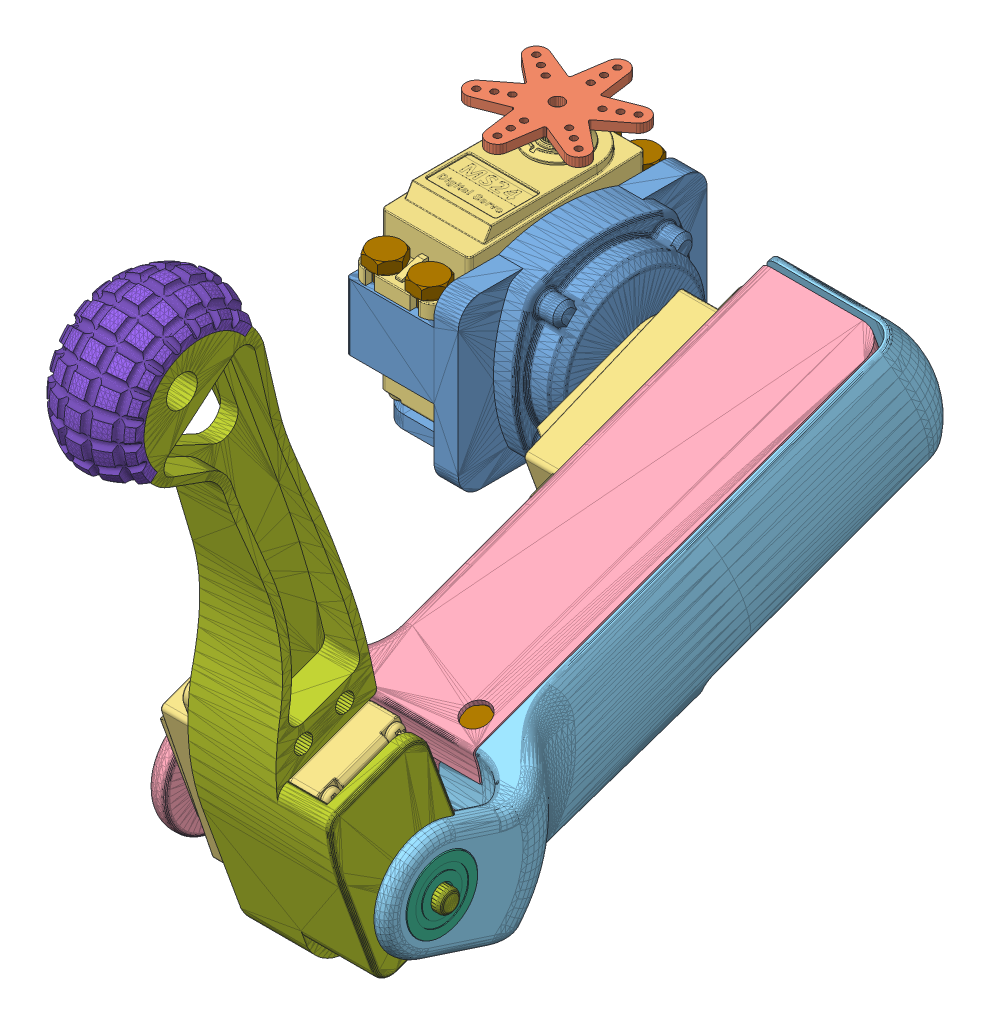
SolidWorks assembly Left Leg Assembly, configuration Default. Lengths in mm.
Overall size (111.25 167.25 201.66).
25 component instances, 9 part files, 58 mates.
Components (placement in the parent):
- Left_arm_joint_mg-1: Left_arm_joint_mg [Default] at (-15.0415 19.5698 -40.5977) size (37.5 46 56.5)
- Servohorn-1: Servohorn [4 Prong] at (19.6585 29.8198 -20.3477) x (0 -0.592234 0.805766) z (-1 0 0) size (31.8 31.8 2.24)
- Servo Motor-1: Servo Motor [Default] at (-5.0415 40.5698 -30.0977) size (20.1 45.99 55.6)
- Servohorn-2: Servohorn [Default] at (-5.0415 60.9698 -30.0977) x (0.506689 0 -0.862129) z (0 -1 0) size (28.18 31.8 2.24)
- Servo Motor-2: Servo Motor [Default] at (38.0585 29.8198 -20.3477) x (0 0.939693 0.34202) z (0 -0.34202 0.939693) size (20.1 45.99 55.6)
- Left_arm_mg-1: Left_arm_mg [Default] at (38.0585 42.7737 -26.7003) x (0 -0.939693 -0.34202) z (0 -0.34202 0.939693) size (38.24 39.8 137.4)
- SM_Left_arm_cover-1: SM_Left_arm_cover [Default] at (38.2585 50.3364 -32.5645) x (0 -0.939693 -0.34202) z (0 -0.34202 0.939693) size (41.16 45 143.55)
- F625ZZ Ball Bearing-1: F625ZZ Ball Bearing [Default] at (78.2585 -1.6568 83.7617) x (0 -0.070361 0.997522) z (-1 0 0) size (18 18 5)
- Servohorn-3: Servohorn [1 Prong] at (28.0585 6.3719 84.4796) x (0 0.893193 -0.449674) z (1 0 0) size (9.55 20.65 2.24)
- Left_wrist_mg-1: Left_wrist_mg [Default] at (18.4585 0.3781 71.7095) x (0 0.939693 0.34202) z (0 -0.34202 0.939693) size (149.99 36.9 30)
- foot-1: foot [Default] at (48.4585 115.3593 124.2008) x (0 0.642788 -0.766044) z (0 -0.766044 -0.642788) size (38.32 20 19.41)
- Servo Motor-3: Servo Motor [Default] at (48.4585 6.3719 84.4796) x (0 0.34202 -0.939693) z (0 0.939693 0.34202) size (20.1 45.99 55.6)
- _Hex_Screws-1: _Hex_Screws [H M4x20] at (-0.0415 43.7698 3.9023) x (-0.837169 0 -0.546944) z (-0.546944 0 0.837169) size (7 22.8 8.08)
- _Hex_Screws-2: _Hex_Screws [H M4x20] at (-10.0415 43.7698 -44.0977) x (-0.837169 0 -0.546944) z (-0.546944 0 0.837169) size (7 22.8 8.08)
- _Hex_Screws-3: _Hex_Screws [H M4x20] at (-10.0415 43.7698 3.9023) x (-0.837169 0 -0.546944) z (-0.546944 0 0.837169) size (7 22.8 8.08)
- _Hex_Screws-4: _Hex_Screws [H M4x20] at (-0.0415 43.7698 -44.0977) x (-0.837169 0 -0.546944) z (-0.546944 0 0.837169) size (7 22.8 8.08)
- _Hex_Screws-5: _Hex_Screws [H M4x20] at (34.8585 22.8895 13.3119) x (0 0.825172 -0.564882) z (0 -0.564882 -0.825172) size (7 22.8 8.08) (hidden)
- _Hex_Screws-6: _Hex_Screws [H M4x20] at (34.8585 13.4926 9.8917) x (0 0.825172 -0.564882) z (0 -0.564882 -0.825172) size (7 22.8 8.08) (hidden)
- _Hex_Screws-7: _Hex_Screws [H M4x20] at (34.8585 39.3065 -31.7933) x (0 0.802845 -0.596188) z (0 -0.596188 -0.802845) size (7 22.8 8.08) (hidden)
- _Hex_Screws-8: _Hex_Screws [H M4x20] at (34.8585 29.9096 -35.2135) x (0 -0.944714 0.327896) z (0 0.327896 0.944714) size (7 22.8 8.08) (hidden)
- _Hex_Screws-9: _Hex_Screws [H M4x20] at (45.2585 40.0315 91.4099) x (0 0.825172 -0.564882) z (0 -0.564882 -0.825172) size (7 22.8 8.08) (hidden)
- _Hex_Screws-10: _Hex_Screws [H M4x20] at (45.2585 36.6113 100.8068) x (0 0.825172 -0.564882) z (0 -0.564882 -0.825172) size (7 22.8 8.08) (hidden)
- _Hex_Screws-11: _Hex_Screws [H M4x20] at (45.2585 -5.0737 74.9929) x (0 0.825172 -0.564882) z (0 -0.564882 -0.825172) size (7 22.8 8.08) (hidden)
- _Hex_Screws-12: _Hex_Screws [H M4x20] at (45.2585 -8.4939 84.3898) x (0 0.825172 -0.564882) z (0 -0.564882 -0.825172) size (7 22.8 8.08) (hidden)
- _Hex_Screws-13: _Hex_Screws [H M3x16] at (62.9617 14.9879 55.4881) x (0.992954 0.04053 -0.111356) z (-0.118503 0.33961 -0.933071) size (5.5 18 6.35)
Mates (geometry in assembly coordinates):
- Coincident4: coincident anti-aligned: plane of Left_arm_joint_mg-1 through (19.6585 19.5698 -40.5977) normal (-1 0 0); plane of Servohorn-1 through (19.6585 29.8198 -20.3477) normal (1 0 0)
- Angle1: planar angle = 0.069813 rad aligned: line of Servohorn-1 through (17.6585 19.7073 -10.6) axis (0 0.470875 -0.8822); line of Left_arm_joint_mg-1 through (4.9585 16.2039 -9.9024) axis (0 0.531268 -0.847204)
- Coincident13: coincident anti-aligned: plane of Left_arm_joint_mg-1 through (4.9585 19.5698 -40.5977) normal (-1 0 0); plane of Servo Motor-1 through (4.9585 51.5698 -1.0977) normal (1 0 0)
- Coincident14: coincident anti-aligned: plane of Left_arm_joint_mg-1 through (-15.0415 19.5698 -0.0977) normal (0 0 -1); plane of Servo Motor-1 through (-15.0415 20.5698 -0.0977) normal (0 0 1)
- Coincident15: coincident anti-aligned: plane of Left_arm_joint_mg-1 through (-15.0415 40.5698 -40.5977) normal (0 1 0); plane of Servo Motor-1 through (3.9585 40.5698 -3.0977) normal (0 -1 0)
- Coincident16: coincident anti-aligned: plane of Servo Motor-1 through (-5.0415 58.9698 -30.0977) normal (0 1 0); plane of Servohorn-2 through (-5.0415 58.9698 -30.0977) normal (0 -1 0)
- Concentric1: concentric aligned: cylinder of Servo Motor-1 through (-5.0415 54.9698 -30.0977) axis (0 1 0) radius 1.25; line of Servohorn-2 through (-5.0415 60.9698 -30.0977) axis (0 1 0)
- Coincident19: coincident aligned: line of Left_arm_joint_mg-1 through (22.4585 29.8198 -20.3477) axis (1 0 0); line of Servohorn-1 through (19.6585 29.8198 -20.3477) axis (1 0 0)
- Concentric3: concentric aligned: line of Servohorn-1 through (19.6585 29.8198 -20.3477) axis (-1 0 0); cylinder of Servo Motor-2 through (23.6585 29.8198 -20.3477) axis (-1 0 0) radius 1.25
- Coincident20: coincident anti-aligned: plane of Servohorn-1 through (19.6585 29.8198 -20.3477) normal (1 0 0); plane of Servo Motor-2 through (19.6585 29.8198 -20.3477) normal (-1 0 0)
- Coincident22: coincident anti-aligned: plane of Left_arm_mg-1 through (38.0585 14.844 50.0357) normal (0 -0.34202 0.939693); plane of SM_Left_arm_cover-1 through (38.2585 19.6373 51.7804) normal (0 0.34202 -0.939693)
- Coincident23: coincident anti-aligned: plane of Left_arm_mg-1 through (38.0585 40.4874 -27.5325) normal (0 -0.939693 -0.34202); plane of SM_Left_arm_cover-1 through (38.2585 43.2568 -35.1413) normal (0 0.939693 0.34202)
- Coincident26: coincident anti-aligned: plane of Servo Motor-2 through (27.0585 29.2981 10.3235) normal (0 0.939693 0.34202); plane of Left_arm_mg-1 through (38.0585 42.7737 -26.7003) normal (0 -0.939693 -0.34202)
- Coincident27: coincident anti-aligned: plane of Servo Motor-2 through (65.5585 10.081 4.4997) normal (0 -0.34202 0.939693); plane of Left_arm_mg-1 through (38.0585 28.9219 11.3572) normal (0 0.34202 -0.939693)
- Coincident28: coincident anti-aligned: plane of Left_arm_mg-1 through (43.0585 42.7737 -26.7003) normal (-1 0 0); plane of SM_Left_arm_cover-1 through (43.0585 50.3364 -32.5645) normal (1 0 0)
- Coincident29: coincident anti-aligned: plane of Servo Motor-2 through (38.0585 29.0424 8.1021) normal (1 0 0); plane of Left_arm_mg-1 through (38.0585 42.7737 -26.7003) normal (-1 0 0)
- Tangent3: tangent anti-aligned: plane of SM_Left_arm_cover-1 through (38.2585 4.6824 76.4813) normal (0 0.148446 0.988921); cylinder of F625ZZ Ball Bearing-1 through (81.2585 6.3233 84.3246) axis (1 0 0) radius 8
- Tangent4: tangent anti-aligned: plane of SM_Left_arm_cover-1 through (38.2585 -0.6707 88.2876) normal (0 0.914236 -0.405181); cylinder of F625ZZ Ball Bearing-1 through (81.2585 6.3233 84.3246) axis (1 0 0) radius 8
- Coincident30: coincident anti-aligned: plane of SM_Left_arm_cover-1 through (79.2585 50.3364 -32.5645) normal (-1 0 0); plane of F625ZZ Ball Bearing-1 through (79.2585 14.3035 84.8875) normal (1 0 0)
- Coincident31: coincident anti-aligned: plane of Left_arm_mg-1 through (30.0585 42.7737 -26.7003) normal (-1 0 0); plane of Servohorn-3 through (30.0585 6.3719 84.4796) normal (1 0 0)
- Coincident33: coincident aligned: line of Left_arm_mg-1 through (30.0585 6.3719 84.4796) axis (-1 0 0); line of Servohorn-3 through (28.0585 6.3719 84.4796) axis (-1 0 0)
- Angle4: planar angle = 0.069813 rad aligned: line of Left_arm_mg-1 through (28.0585 -1.5315 69.0529) axis (0 0.180422 0.983589); line of Servohorn-3 through (28.0585 0.3586 80.1572) axis (0 0.248594 0.968608)
- Coincident44: coincident aligned: plane of Left_wrist_mg-1 through (68.4585 0.3781 71.7095) normal (1 0 0); plane of foot-1 through (68.4585 115.3593 124.2008) normal (1 0 0)
- Coincident52: coincident anti-aligned: plane of Left_wrist_mg-1 through (18.4585 93.6986 150.0149) normal (0 0.766044 0.642788); plane of foot-1 through (48.4585 115.3593 124.2008) normal (0 -0.766044 -0.642788)
- Coincident54: coincident: line of Left_wrist_mg-1 through (68.4585 125.3177 132.5572) axis (0 -0.687865 0.725839); point of foot-1
- Coincident55: coincident anti-aligned: plane of Left_wrist_mg-1 through (18.4585 -6.4623 90.5034) normal (0 0.34202 -0.939693); plane of Servo Motor-3 through (75.9585 -6.5563 90.4691) normal (0 -0.34202 0.939693)
- Coincident56: coincident anti-aligned: plane of Left_wrist_mg-1 through (18.4585 0.3781 71.7095) normal (0 0.939693 0.34202); plane of Servo Motor-3 through (68.4585 -6.4452 90.4564) normal (0 -0.939693 -0.34202)
- Coincident57: coincident anti-aligned: plane of Left_wrist_mg-1 through (48.4585 0.3781 71.7095) normal (-1 0 0); plane of Servo Motor-3 through (48.4585 34.8218 85.257) normal (1 0 0)
- Concentric4: concentric aligned: line of Servohorn-3 through (28.0585 6.3719 84.4796) axis (-1 0 0); cylinder of Servo Motor-3 through (34.0585 6.3719 84.4796) axis (-1 0 0) radius 1.25
- Coincident58: coincident anti-aligned: plane of Servohorn-3 through (30.0585 6.3719 84.4796) normal (1 0 0); plane of Servo Motor-3 through (30.0585 6.3719 84.4796) normal (-1 0 0)
- Concentric5: concentric aligned: cylinder of Servo Motor-1 through (-0.0415 34.2058 3.9023) axis (0 1 0) radius 2.25; cylinder of _Hex_Screws-1 through (-0.0415 23.7698 3.9023) axis (0 1 0) radius 2
- Concentric6: concentric aligned: cylinder of Servo Motor-1 through (-10.0415 34.2058 3.9023) axis (0 1 0) radius 2.25; cylinder of _Hex_Screws-3 through (-10.0415 23.7698 3.9023) axis (0 1 0) radius 2
- Concentric7: concentric aligned: cylinder of Servo Motor-1 through (-0.0415 34.2058 -44.0977) axis (0 1 0) radius 2.25; cylinder of _Hex_Screws-4 through (-0.0415 23.7698 -44.0977) axis (0 1 0) radius 2
- Concentric8: concentric aligned: cylinder of Servo Motor-1 through (-10.0415 34.2058 -44.0977) axis (0 1 0) radius 2.25; cylinder of _Hex_Screws-2 through (-10.0415 23.7698 -44.0977) axis (0 1 0) radius 2
- Coincident59: coincident aligned: plane of Servo Motor-1 through (-5.0415 43.7698 -30.0977) normal (0 1 0); circle of _Hex_Screws-2
- Coincident60: coincident anti-aligned: plane of Servo Motor-1 through (-5.0415 43.7698 -30.0977) normal (0 1 0); plane of _Hex_Screws-4 through (-0.0415 43.7698 -44.0977) normal (0 -1 0)
- Coincident61: coincident anti-aligned: plane of Servo Motor-1 through (-5.0415 43.7698 -30.0977) normal (0 1 0); plane of _Hex_Screws-1 through (-0.0415 43.7698 3.9023) normal (0 -1 0)
- Coincident62: coincident anti-aligned: plane of Servo Motor-1 through (-5.0415 43.7698 -30.0977) normal (0 1 0); plane of _Hex_Screws-3 through (-10.0415 43.7698 3.9023) normal (0 -1 0)
- Concentric9: concentric aligned: cylinder of Servo Motor-2 through (44.4225 22.8895 13.3119) axis (-1 0 0) radius 2.25; cylinder of _Hex_Screws-5 through (54.8585 22.8895 13.3119) axis (-1 0 0) radius 2
- Concentric10: concentric aligned: cylinder of Servo Motor-2 through (44.4225 13.4926 9.8917) axis (-1 0 0) radius 2.25; cylinder of _Hex_Screws-6 through (54.8585 13.4926 9.8917) axis (-1 0 0) radius 2
- Concentric11: concentric aligned: cylinder of Servo Motor-2 through (44.4225 39.3065 -31.7933) axis (-1 0 0) radius 2.25; cylinder of _Hex_Screws-7 through (54.8585 39.3065 -31.7933) axis (-1 0 0) radius 2
- Concentric12: concentric aligned: cylinder of Servo Motor-2 through (44.4225 29.9096 -35.2135) axis (-1 0 0) radius 2.25; cylinder of _Hex_Screws-8 through (54.8585 29.9096 -35.2135) axis (-1 0 0) radius 2
- Coincident63: coincident anti-aligned: plane of Servo Motor-2 through (34.8585 29.8198 -20.3477) normal (-1 0 0); plane of _Hex_Screws-8 through (34.8585 29.9096 -35.2135) normal (1 0 0)
- Coincident64: coincident anti-aligned: plane of Servo Motor-2 through (34.8585 29.8198 -20.3477) normal (-1 0 0); plane of _Hex_Screws-7 through (34.8585 39.3065 -31.7933) normal (1 0 0)
- Coincident65: coincident anti-aligned: plane of Servo Motor-2 through (34.8585 29.8198 -20.3477) normal (-1 0 0); plane of _Hex_Screws-5 through (34.8585 22.8895 13.3119) normal (1 0 0)
- Coincident66: coincident anti-aligned: plane of Servo Motor-2 through (34.8585 29.8198 -20.3477) normal (-1 0 0); plane of _Hex_Screws-6 through (34.8585 13.4926 9.8917) normal (1 0 0)
- Concentric13: concentric aligned: cylinder of Servo Motor-3 through (54.8225 36.6113 100.8068) axis (-1 0 0) radius 2.25; cylinder of _Hex_Screws-10 through (65.2585 36.6113 100.8068) axis (-1 0 0) radius 2
- Concentric14: concentric aligned: cylinder of Servo Motor-3 through (54.8225 40.0315 91.4099) axis (-1 0 0) radius 2.25; cylinder of _Hex_Screws-9 through (65.2585 40.0315 91.4099) axis (-1 0 0) radius 2
- Concentric15: concentric aligned: cylinder of Servo Motor-3 through (54.8225 -5.0737 74.9929) axis (-1 0 0) radius 2.25; cylinder of _Hex_Screws-11 through (65.2585 -5.0737 74.9929) axis (-1 0 0) radius 2
- Concentric16: concentric aligned: cylinder of Servo Motor-3 through (54.8225 -8.4939 84.3898) axis (-1 0 0) radius 2.25; cylinder of _Hex_Screws-12 through (65.2585 -8.4939 84.3898) axis (-1 0 0) radius 2
- Coincident67: coincident anti-aligned: plane of Servo Motor-3 through (45.2585 6.3719 84.4796) normal (-1 0 0); plane of _Hex_Screws-11 through (45.2585 -5.0737 74.9929) normal (1 0 0)
- Coincident68: coincident anti-aligned: plane of Servo Motor-3 through (45.2585 6.3719 84.4796) normal (-1 0 0); plane of _Hex_Screws-10 through (45.2585 36.6113 100.8068) normal (1 0 0)
- Coincident69: coincident anti-aligned: plane of Servo Motor-3 through (45.2585 6.3719 84.4796) normal (-1 0 0); plane of _Hex_Screws-9 through (45.2585 40.0315 91.4099) normal (1 0 0)
- Coincident70: coincident anti-aligned: plane of Left_arm_mg-1 through (38.0585 44.6531 -26.0163) normal (0 0.939693 0.34202); plane of _Hex_Screws-13 through (62.9617 14.9879 55.4881) normal (0 -0.939693 -0.34202)
- Tangent5: tangent anti-aligned: plane of Left_arm_mg-1 through (27.0618 14.2077 51.7841) normal (0.130537 0.339094 -0.931652); cylinder of _Hex_Screws-13 through (62.9617 -0.0472 50.0157) axis (0 0.939693 0.34202) radius 1.5
- Tangent6: tangent anti-aligned: plane of Left_arm_mg-1 through (72.2748 41.233 -22.4673) normal (0.991445 -0.044643 0.122657); cylinder of _Hex_Screws-13 through (62.9617 -0.0472 50.0157) axis (0 0.939693 0.34202) radius 1.5
- Angle5: planar angle = 0.349066 rad aligned: plane of Left_arm_mg-1 through (38.0585 45.5099 -34.2179) normal (0 0.34202 -0.939693); plane of Left_arm_joint_mg-1 through (-15.0415 19.5698 -48.5977) normal (0 0 -1)
- Angle6: planar angle = 1.570796 rad anti-aligned: plane of Servo Motor-3 through (37.4585 37.0432 85.0013) normal (0 0.34202 -0.939693); plane of Left_arm_mg-1 through (38.0585 47.4722 -24.9902) normal (0 0.939693 0.34202)
